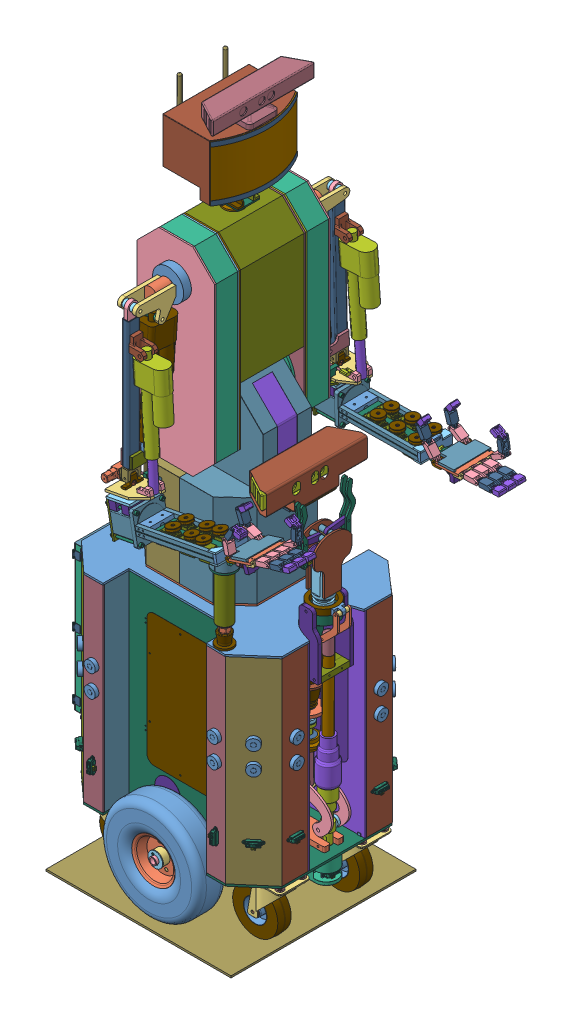
SolidWorks assembly sorbot, configuration По умолчанию. Lengths in mm. (continued)
Components (placement in the parent): (continued)
- pillar.10mm-9: pillar.10mm [Default] at (211.9932 95.4897 -58.2424) x (-0.73854 -0.67421 0) z (-0.67421 0.73854 0) size (7 10 7)
- pillar.10mm-10: pillar.10mm [Default] at (212.0094 150.4897 -58.2424) x (-0.73854 -0.67421 0) z (-0.67421 0.73854 0) size (7 10 7)
- platform.motor.drivers-1: platform.motor.drivers [Default] at (80.8907 152.4914 -189.9653) x (0 0 1) z (-1 0 0) size (159.34 76.47 117)
  - dirvers.motor.assembly-1: dirvers.motor.assembly [Default] at (49.223 64.9012 121.2019) size (145 32 117)
  - pillar.10mm-1: pillar.10mm [Default] at (-13.277 69.9012 103.7019) size (7 10 7)
  - vnh2sp30-1: vnh2sp30 [Default] at (2.7293 79.9012 115.4439) size (38 1.5 30)
  - pillar.10mm-2: pillar.10mm [Default] at (18.6548 69.9012 103.7019) size (7 10 7)
  - pillar.10mm-3: pillar.10mm [Default] at (18.6548 69.9012 127.4284) size (7 10 7)
  - pillar.10mm-4: pillar.10mm [Default] at (27.723 69.9012 103.7019) size (7 10 7)
  - vnh2sp30-2: vnh2sp30 [Default] at (43.7293 79.9012 115.4439) size (38 1.5 30)
  - pillar.10mm-5: pillar.10mm [Default] at (59.6548 69.9012 103.7019) size (7 10 7)
  - pillar.10mm-6: pillar.10mm [Default] at (59.6548 69.9012 127.4284) size (7 10 7)
  - pillar.10mm-7: pillar.10mm [Default] at (70.723 69.9012 103.7019) size (7 10 7)
  - vnh2sp30-3: vnh2sp30 [Default] at (86.7293 79.9012 115.4439) size (38 1.5 30)
  - pillar.10mm-8: pillar.10mm [Default] at (102.6548 69.9012 103.7019) size (7 10 7)
  - pillar.10mm-9: pillar.10mm [Default] at (102.6548 69.9012 127.4284) size (7 10 7)
  - fan1.fixture-1: fan1.fixture [Default] at (106.723 64.9012 93.8312) size (16.5 71.5 44)
  - PC Fan-1: PC Fan [Default] at (71.3146 136.8013 172.3383) x (0 -1 0) z (0 0 1) size (47.91 13.68 47.91)
    - Fan - housing-1: Fan - housing [Default] at (23.3881 57.9083 -56.6715) x (0 -1 0) z (-1 0 0) size (13.68 37 37)
    - Fan - propeller-1: Fan - propeller [Default] at (23.3881 58.6083 -56.6715) x (-0.764125 0 -0.645068) z (0 1 0) size (34 34 7.89)
  - radiator1-1: radiator1 [Default] at (2.2293 83.4012 115.4439) x (0 0 1) z (-1 0 0) size (47 23 17)
  - radiator2-1: radiator2 [Default] at (43.7293 83.4012 115.4439) x (0 0 1) z (-1 0 0) size (60 39 27)
  - radiator2-2: radiator2 [Default] at (86.7293 83.4012 115.4439) x (0 0 1) z (-1 0 0) size (60 39 27)
  - screw.m4x35-1: screw.m4x35 [Default] at (4.1241 64.9012 94.8432) size (10.8 29 10.8)
  - screw.m4x35-2: screw.m4x35 [Default] at (4.1241 64.9012 136.0446) size (10.8 29 10.8)
  - screw.m4x35-3: screw.m4x35 [Default] at (45.6241 64.9012 88.5829) size (10.8 29 10.8)
  - screw.m4x35-4: screw.m4x35 [Default] at (45.6241 64.9012 142.3048) size (10.8 29 10.8)
  - screw.m4x35-5: screw.m4x35 [Default] at (88.6241 64.9012 88.5829) size (10.8 29 10.8)
  - screw.m4x35-6: screw.m4x35 [Default] at (88.6241 64.9012 142.3048) size (10.8 29 10.8)
- computer.box.screw.fixture-5: computer.box.screw.fixture [Default] at (-89.5362 420.1505 8.4522) x (0 1 0) z (-1 0 0) size (25 10 10)
- computer.box.screw.fixture-6: computer.box.screw.fixture [Default] at (-89.5362 260.1505 8.4522) x (0 -1 0) z (1 0 0) size (25 10 10)
- computer.box.screw.fixture-7: computer.box.screw.fixture [Default] at (75.4638 420.1505 8.4522) x (0 -1 0) z (1 0 0) size (25 10 10)
- computer.box.screw.fixture-8: computer.box.screw.fixture [Default] at (75.4638 260.1505 8.4522) x (0 -1 0) z (1 0 0) size (25 10 10)
- computer.box.screw.fixture-9: computer.box.screw.fixture [Default] at (-7.0362 175.1505 8.4522) x (1 0 0) z (0 1 0) size (25 10 10)
- computer.box.screw.fixture-10: computer.box.screw.fixture [Default] at (-7.0362 505.1505 8.4522) x (1 0 0) z (0 1 0) size (25 10 10)
- computer.box.screw.fixture-11: computer.box.screw.fixture [Default] at (-6.9656 175.1505 -282.1821) x (1 0 0) z (0 -1 0) size (25 10 10)
- computer.box.screw.fixture-12: computer.box.screw.fixture [Default] at (75.5344 420.1505 -282.1821) x (0 1 0) z (1 0 0) size (25 10 10)
- computer.box.screw.fixture-13: computer.box.screw.fixture [Default] at (-6.9656 505.1505 -282.1821) x (1 0 0) z (0 -1 0) size (25 10 10)
- computer.box.screw.fixture-14: computer.box.screw.fixture [Default] at (75.5344 260.1505 -282.1821) x (0 1 0) z (1 0 0) size (25 10 10)
- computer.box.screw.fixture-15: computer.box.screw.fixture [Default] at (-89.4656 260.1505 -282.1821) x (0 1 0) z (1 0 0) size (25 10 10)
- computer.box.screw.fixture-16: computer.box.screw.fixture [Default] at (-89.4656 420.1505 -282.1821) x (0 1 0) z (1 0 0) size (25 10 10)
- plates.fixture-1: plates.fixture [Default] at (-94.2054 480.3702 -281.1821) x (0 0 1) z (-1 0 0) size (18.98 21 15)
- plates.fixture-2: plates.fixture [Default] at (-94.2054 228.5986 -281.1821) x (0 0 1) z (-1 0 0) size (18.98 21 15)
- left.plate-1: left.plate [Default] at (-11.6361 340.1505 -239.559) x (1 0 0) z (0 1 0) size (150 2 294)
- plates.fixture-3: plates.fixture [Default] at (-66.9634 476.3702 -242.559) x (0 0 -1) z (-1 0 0) size (18.98 21 15)
- plates.fixture-4: plates.fixture [Default] at (-66.9634 224.5986 -242.559) x (0 0 -1) z (-1 0 0) size (18.98 21 15)
- plate.console-1: plate.console [Default] at (-43.3033 477.3702 -231.7221) x (-0.961017 0 -0.276489) z (0.276489 0 -0.961017) size (44.8 2 28.3)
- plate.console-2: plate.console [Default] at (-43.3033 225.5986 -231.7221) x (-0.961017 0 -0.276489) z (0.276489 0 -0.961017) size (44.8 2 28.3)
- right.plate-1: right.plate [Default] at (-9.2671 340.1505 -29.4493) x (1 0 0) z (0 -1 0) size (150 2 294)
- plates.fixture-5: plates.fixture [Default] at (-109.2054 480.3702 7.4522) x (0 0 -1) z (1 0 0) size (18.98 21 15)
- plates.fixture-6: plates.fixture [Default] at (-109.2054 228.5986 7.4522) x (0 0 -1) z (1 0 0) size (18.98 21 15)
- plate.console-3: plate.console [Default] at (-37.759 479.3702 -31.8467) x (-0.993461 0 0.11417) z (0.11417 0 0.993461) size (44.8 2 28.3)
- plate.console-4: plate.console [Default] at (-37.759 227.5986 -31.8467) x (-0.993461 0 0.11417) z (0.11417 0 0.993461) size (44.8 2 28.3)
- plates.fixture-7: plates.fixture [Default] at (-79.5944 476.3702 -26.4493) x (0 0 1) z (1 0 0) size (18.98 21 15)
- plates.fixture-8: plates.fixture [Default] at (-79.5944 224.5986 -26.4493) x (0 0 1) z (1 0 0) size (18.98 21 15)
- us_sesnor_board-5: us_sesnor_board [Default] at (156.7984 270.4368 -340.1821) x (0 -1 0) z (-1 0 0) size (57 1.5 32)
- us_sesnor_board-6: us_sesnor_board [Default] at (208.5725 230.4368 -317.4683) x (0 1 0) z (0.759435 0 0.650583) size (57 1.5 32)
- us_sesnor_board-7: us_sesnor_board [Default] at (251.2324 210.4368 -249.3603) x (0 1 0) z (0.00186 0 0.999998) size (57 1.5 32)
- us_sesnor_board-8: us_sesnor_board [Default] at (251.1742 210.4368 -22.2417) x (0 1 0) z (0 0 1) size (57 1.5 32)
- us_sesnor_board-9: us_sesnor_board [Default] at (206.521 230.4368 45.4742) x (0 1 0) z (-0.759435 0 0.650583) size (57 1.5 32)
- us_sesnor_board-10: us_sesnor_board [Default] at (159.7428 270.4368 66.4522) x (0 -1 0) z (1 0 0) size (57 1.5 32)
- pillar.10mm-11: pillar.10mm [Default] at (143.5283 296.7164 -350.1821) x (0 -1 0) z (-1 0 0) size (7 10 7)
- pillar.10mm-12: pillar.10mm [Default] at (169.3356 244.6047 -350.1821) x (0 -1 0) z (-1 0 0) size (7 10 7)
- pillar.10mm-13: pillar.10mm [Default] at (225.1561 204.1572 -316.4293) x (0 1 0) z (0.759435 0 0.650583) size (7 10 7)
- pillar.10mm-14: pillar.10mm [Default] at (205.5571 256.2689 -333.2192) x (0 1 0) z (0.759435 0 0.650583) size (7 10 7)
- pillar.10mm-15: pillar.10mm [Default] at (261.2571 184.1572 -236.1088) x (0 1 0) z (0.00186 0 0.999998) size (7 10 7)
- pillar.10mm-16: pillar.10mm [Default] at (261.2091 236.2689 -261.9161) x (0 1 0) z (0.00186 0 0.999998) size (7 10 7)
- pillar.10mm-17: pillar.10mm [Default] at (261.1742 236.2689 -34.779) x (0 1 0) z (0 0 1) size (7 10 7)
- pillar.10mm-18: pillar.10mm [Default] at (261.1742 184.1572 -8.9716) x (0 1 0) z (0 0 1) size (7 10 7)
- pillar.10mm-19: pillar.10mm [Default] at (202.949 204.1572 61.7019) x (0 1 0) z (-0.759435 0 0.650583) size (7 10 7)
- pillar.10mm-20: pillar.10mm [Default] at (222.548 256.2689 44.9121) x (0 1 0) z (-0.759435 0 0.650583) size (7 10 7)
- pillar.10mm-21: pillar.10mm [Default] at (173.0129 296.7164 76.4522) x (0 -1 0) z (1 0 0) size (7 10 7)
- pillar.10mm-22: pillar.10mm [Default] at (147.2055 244.6047 76.4522) x (0 -1 0) z (1 0 0) size (7 10 7)
- acdc.220V.filter-1: acdc.220V.filter [Default] at (235.8821 406.6863 -46.2424) x (0 1 0) z (1 0 0) size (297.85 43 50)
- pillar.10mm-23: pillar.10mm [Default] at (235.8821 551.7681 -46.2424) x (0 -1 0) z (1 0 0) size (7 10 7)
- pillar.10mm-24: pillar.10mm [Default] at (235.8821 261.6046 -46.2424) x (-0.028691 -0.999588 0) z (0.999588 -0.028691 0) size (7 10 7)
- acdc.12v.power.supply-1: acdc.12v.power.supply [Default] at (169.7521 152.7755 -317.8791) x (0 1 0) z (0 0 -1) size (125 30 50)
- AC-DC-12-fixture-1: AC-DC-12-fixture [Default] at (138.7521 154.3322 -328.3791) x (0 0 1) z (0 1 0) size (24.5 56.75 30.18)
- AC-DC-12-fixture-2: AC-DC-12-fixture [Default] at (138.7521 154.3322 -307.3791) x (0 0 -1) z (0 -1 0) size (24.5 56.75 30.18)
- encoder-2-1: encoder-2 [Default] at (-6.6918 11.9368 -256.3681) x (1 0 0) z (0 -1 0) size (68 0.5 68)
- encoder-2-2: encoder-2 [Default] at (-6.6918 11.9368 -16.3681) x (1 0 0) z (0 -1 0) size (68 0.5 68)
- spool.220v-1: spool.220v [Default] at (27.3222 599.5624 89.7858) x (0 0 -1) z (0 -1 0) size (136.63 47 130)
  - spool.ac220v.base-1: spool.ac220v.base [Default] at (13.3335 111.5787 102.4119) size (136.63 5 130)
  - spool.220vac.spool.base.p1-1: spool.220vac.spool.base.p1 [Default] at (88.3335 116.5787 167.4119) size (121 5 121)
  - spool.disk.p1-1: spool.disk.p1 [Default] at (88.3335 121.5787 167.4119) size (121 1.5 121)
  - spool.disk2.pillar-1: spool.disk2.pillar [Default] at (141.3335 123.0787 167.4119) size (9 27 9)
  - spool.disk2.pillar-2: spool.disk2.pillar [Default] at (88.3335 123.0787 220.4119) size (9 27 9)
  - spool.disk2.pillar-3: spool.disk2.pillar [Default] at (35.3335 123.0787 167.4119) size (9 27 9)
  - spool.disk2.pillar-4: spool.disk2.pillar [Default] at (88.3335 123.0787 114.4119) size (9 27 9)
  - spool.disk.p2-1: spool.disk.p2 [Default] at (88.3335 150.0787 167.4119) size (121 1.5 121)
  - screw.m4x40-1: screw.m4x40 [Default] at (88.3335 118.5787 220.4119) x (-0.837169 0 -0.546944) z (-0.546944 0 0.837169) size (10 42 10)
  - screw.m4x40-2: screw.m4x40 [Default] at (141.3335 118.5787 167.4119) x (-0.837169 0 -0.546944) z (-0.546944 0 0.837169) size (10 42 10)
  - screw.m4x40-3: screw.m4x40 [Default] at (88.3335 118.5787 114.4119) x (-0.837169 0 -0.546944) z (-0.546944 0 0.837169) size (10 42 10)
  - screw.m4x40-4: screw.m4x40 [Default] at (35.3335 118.5787 167.4119) x (-0.837169 0 -0.546944) z (-0.546944 0 0.837169) size (10 42 10)
  - m4.nut-1: m4.nut [По умолчанию] at (141.3335 151.5787 167.4119) size (6.86 5 7.92)
  - m4.nut-2: m4.nut [По умолчанию] at (35.3335 151.5787 167.4119) size (6.86 5 7.92)
  - m4.nut-3: m4.nut [По умолчанию] at (88.3335 151.5787 114.4119) size (6.86 5 7.92)
  - m4.nut-4: m4.nut [По умолчанию] at (88.3335 151.5787 220.4119) size (6.86 5 7.92)
- wall2.cap-1: wall2.cap [Default] at (136.6115 375.4739 -212.2424) x (1 0 0) z (0 -1 0) size (170 0.5 350)
- wall2.cap-2: wall2.cap [Default] at (136.1134 375.6582 -62.2424) x (1 0 0) z (0 1 0) size (170 0.5 350)
- spool.220v.inlet-1: spool.220v.inlet [Default] at (160.9714 590.1505 61.3093) size (44 32.78 44)
- charger.module-1: charger.module [Default] at (132.5657 748.9564 17.9664) x (0.996526 0 -0.083283) z (0.083283 0 0.996526) size (60 284.68 60)
  - charger.module.base.p2-1: charger.module.base.p2 [Default] at (24.6973 28.3142 45.5581) size (59 10 59)
  - charger.module.case.p1-1: charger.module.case.p1 [Default] at (24.6973 38.3142 45.5581) size (59 22.9 59)
  - charger.module.camera-1: charger.module.camera [Default] at (24.6973 39.9144 45.5581) x (0.99995 0 0.009956) z (-0.009956 0 0.99995) size (34.64 19.2 34.64)
  - charger.module.motor.fixture-1: charger.module.motor.fixture [Default] at (24.6973 61.2142 45.5581) size (59 0.5 59)
  - charger.module.case.p2-1: charger.module.case.p2 [Default] at (24.6973 61.7142 45.5581) size (59 15 59)
  - charger.module.plug.p1-1: charger.module.plug.p1 [Default] at (24.6973 50.9902 45.5581) x (0.996646 0 0.081829) z (-0.081829 0 0.996646) size (32 40 32)
  - charger.module.motor-1: charger.module.motor [Default] at (46.1037 37.2096 54.3775) x (0.391862 0 -0.920024) z (0.920024 0 0.391862) size (12 35.5 10)
  - charger.module.gear.p1-1: charger.module.gear.p1 [Default] at (24.6973 67.2142 45.5581) x (0.999921 0 0.012536) z (-0.012536 0 0.999921) size (36.8 4.5 36.8)
  - charger.module.gear.p2-1: charger.module.gear.p2 [Default] at (46.1037 67.7096 54.3775) x (1 0 -0.000212) z (0.000212 0 1) size (11 8 11)
  - charger.module.insulation.p1-1: charger.module.insulation.p1 [Default] at (24.6973 63.7142 45.5581) x (0.996646 0 0.081829) z (-0.081829 0 0.996646) size (30 4 30)
  - charger.module.contact-1: charger.module.contact [Default] at (24.6973 58.7142 45.5581) size (30 5 30)
  - charger.module.insulation.p2-1: charger.module.insulation.p2 [Default] at (24.6973 56.7142 45.5581) x (0.996646 0 0.081829) z (-0.081829 0 0.996646) size (30 2 30)
  - charger.module.contact-2: charger.module.contact [Default] at (24.6973 51.7142 45.5581) size (30 5 30)
  - charger.module.insulation.p3-1: charger.module.insulation.p3 [Default] at (24.6973 49.2142 45.5581) size (30 2.5 30)
  - charger.module.cover-1: charger.module.cover [Default] at (24.6973 28.7142 45.5581) size (60 48 60)
  - charger.module.aluminum.base-1: charger.module.aluminum.base [Default] at (24.6973 23.3142 45.5581) size (59 32 59)
  - charger.module.handle-1: charger.module.handle [Default] at (24.6973 -104.6858 45.5581) size (40 128 40)
  - charger.module.cap-1: charger.module.cap [Default] at (24.6973 -107.1858 45.5581) size (38 14.5 38)
  - charger.module.cable.inlet.nut-1: charger.module.cable.inlet.nut [Default] at (24.6973 -104.6858 45.5581) x (0.829784 0 0.558085) z (-0.558085 0 0.829784) size (23.82 5 22.58)
  - charger.module.cable.inlet.nut.external-1: charger.module.cable.inlet.nut.external [Default] at (24.6973 -107.1858 45.5581) x (-0.837169 0 -0.546944) z (-0.546944 0 0.837169) size (25.34 15 22.82)
  - charger.module.cable.inlet.tail-1: charger.module.cable.inlet.tail [Default] at (24.6973 -114.1858 45.5581) x (-0.837169 0 -0.546944) z (-0.546944 0 0.837169) size (25.34 60 22.82)
- scanning.distance.meter.platform.bottom-1: scanning.distance.meter.platform.bottom [Default] at (253.6127 48.5992 -170.4978) x (-1 0 0) z (0 0 1) size (55.5 60.35 60)
  - servo.sm-s3317s-1: servo.sm-s3317s [Default] at (17.6103 2.1624 33.6342) size (42 32.4 16.3)
  - Sharp IR GP2D120-1: Sharp IR GP2D120 [Predeterminado] at (-1.2396 42.2544 36.8712) x (0 0 1) z (-1 0 0) size (44.5 19 13.9)
    - Sharp IR Body-1: Sharp IR Body [Predeterminado] at (-3.237 2.158 -6.95) size (44.5 13 13.9)
    - Sharp IR JST-1: Sharp IR JST [Predeterminado] at (-3.237 2.158 -3.95) size (28 18 7)
  - servo-sms3317s-lever-1: servo-sms3317s-lever [Default] at (9.4603 35.7624 33.6342) x (0 0 -1) z (-1 0 0) size (37.37 4.4 7)
  - scanning.distance.meter.sensor.fixture-1: scanning.distance.meter.sensor.fixture [Default] at (5.7103 36.1624 10.6342) size (7.5 15 46)
  - scanning.distance.meter.case-1: scanning.distance.meter.case [Default] at (11.0014 62.5124 33.6342) size (55.5 60.35 60)
- kinect-1: kinect [По умолчанию] at (202.8758 910.3423 -136.6669) x (0 0 1) z (-1 0 0) size (276 72 65)
- body.cover.glass-1: body.cover.glass [Default] at (129.0303 942.6564 -137.0438) x (0 0 1) z (-1 0 0) size (79.82 175.77 79.37)
- frontal.kinect.plate-1: frontal.kinect.plate [Default] at (172.5303 854.8423 -136.6669) x (0 0 -1) z (1 0 0) size (120 2 80)
- frontal.kinect.plate.fixture-1: frontal.kinect.plate.fixture [Default] at (134.0303 854.8423 -96.6669) x (0 1 0) z (1 0 0) size (40 20 66.5)
- frontal.kinect.plate.fixture-2: frontal.kinect.plate.fixture [Default] at (134.0303 854.8423 -196.6669) x (0 1 0) z (1 0 0) size (40 20 66.5)
- frontal.kinect.cover-1: frontal.kinect.cover [Default] at (172.5303 857.3423 -136.6669) x (0 0 -1) z (1 0 0) size (272 81 81)
- body.cover.back-1: body.cover.back [По умолчанию] at (-55.0648 1082.7934 -136.9735) x (0 0 1) z (-1 0 0) size (278.72 470.5 152.62)
- back.camera.housing-1: back.camera.housing [Default] at (-158.0178 1016.2961 -137.3735) x (0 0 1) z (-0.707107 -0.707107 0) size (92.1 36.15 55.95)
Mates (geometry in assembly coordinates):
- Концентричный1: concentric anti-aligned: cylinder of wheel-2/wheel.metal.internal-1 through (-6.6918 11.9368 -351.3681) axis (0 0 1) radius 10; cylinder of wheel-1/wheel.metal.internal-1 through (-6.6918 11.9368 79.1319) axis (0 0 -1) radius 10
- Концентричный2: concentric anti-aligned: cylinder of wheel-1/wheel.metal.internal-1 through (-6.6918 11.9368 79.1319) axis (0 0 -1) radius 10; cylinder of wheel.axis-1 through (-6.6918 11.9368 -361.8681) axis (0 0 1) radius 10
- Концентричный3: concentric anti-aligned: cylinder of wheel.axis-1 through (-6.6918 11.9368 -361.8681) axis (0 0 1) radius 10; cylinder of wheel.washer-1 through (-6.6918 11.9368 81.1319) axis (0 0 -1) radius 10
- Совпадение3: coincident anti-aligned: plane of wheel-1/wheel.metal.internal-1 through (-6.6918 11.9368 79.1319) normal (0 0 1); plane of wheel.washer-1 through (-6.6918 11.9368 79.1319) normal (0 0 -1)
- Концентричный4: concentric anti-aligned: cylinder of wheel.axis-1 through (-6.6918 11.9368 -361.8681) axis (0 0 1) radius 10; cylinder of wheel.washer-2 through (-6.6918 11.9368 -351.3681) axis (0 0 -1) radius 10
- Совпадение4: coincident anti-aligned: plane of wheel.washer-2 through (-6.6918 11.9368 -351.3681) normal (0 0 1); plane of wheel-2/wheel.metal.internal-1 through (-6.6918 11.9368 -351.3681) normal (0 0 -1)
- Параллельность1: parallel aligned: line of wheel.axis-1 through (0.9691 -6.5378 -355.8681) axis (-0.383049 0.923728 0); circle of wheel.axis.splint-2
- Концентричный5: concentric aligned: cylinder of wheel-2/wheel.metal.internal-1 through (-6.6918 11.9368 -291.3681) axis (0 0 -1) radius 19; cylinder of wheel.disk-1 through (-6.6918 11.9368 -311.3681) axis (0 0 -1) radius 18.9
- Совпадение7: coincident anti-aligned: plane of wheel-2/wheel.metal.internal-1 through (-25.4032 15.2361 -326.3681) normal (0 0 1); plane of wheel.disk-1 through (-6.6918 11.9368 -326.3681) normal (0 0 -1)
- Концентричный6: concentric anti-aligned: cylinder of wheel.axis-1 through (-6.6918 11.9368 -361.8681) axis (0 0 1) radius 10; cylinder of wheel.bearing-1 through (-6.6918 11.9368 -256.3681) axis (0 0 -1) radius 10
- Концентричный8: concentric aligned: cylinder of wheel.axis-1 through (-6.6918 11.9368 -361.8681) axis (0 0 1) radius 10; cylinder of wheel.stop.bearing-2/wheel.stop.bearing.p1-2 through (-6.6918 11.9368 -246.3457) axis (0 0 1) radius 10
- Совпадение10: coincident anti-aligned: plane of wheel.disk-1 through (-6.6918 11.9368 -256.3681) normal (0 0 1); plane of wheel.stop.bearing-2/wheel.stop.bearing.p1-1 through (-6.6918 11.9368 -256.3681) normal (0 0 -1)
- Концентричный10: concentric anti-aligned: cylinder of gearmotor-1 through (53.2168 119.2767 -284.0001) axis (0 0 1) radius 7; cylinder of gearmotor.sprocket.wheel.disk-1 through (53.2168 119.2767 -217.7117) axis (0 0 -1) radius 7
- Концентричный13: concentric anti-aligned: cylinder of wheel.axis-1 through (-6.6918 11.9368 -361.8681) axis (0 0 1) radius 10; cylinder of sprocket-1 through (-6.6918 11.9368 -268.3681) axis (0 0 -1) radius 26
- Концентричный14: concentric anti-aligned: circle of gearmotor-1; circle of sproket.initial-1
- Совпадение16: coincident aligned: plane of sproket.initial-1 through (64.3825 152.5534 -268.5001) normal (0 0 1); circle of gearmotor.sprocket.wheel.disk-1
- Параллельность2: parallel anti-aligned: plane of sproket.initial-1 through (64.3825 152.5534 -271.5001) normal (0 0 -1); plane of sprocket-1 through (4.6992 45.137 -268.3681) normal (0 0 1)
- Совпадение57: coincident anti-aligned: plane of sprocket-1 through (4.6992 45.137 -271.3681) normal (0 0 -1); plane of wheel.disk-1 through (-6.6918 11.9368 -271.3681) normal (0 0 1)
- Совпадение61: coincident anti-aligned: plane of gearmotor-1 through (53.2168 119.2767 -254.0001) normal (0 0 -1); plane of gearmotor.sprocket.wheel.disk-1 through (53.2168 119.2767 -254.0001) normal (0 0 1)
- Параллельность3: parallel aligned: plane of sproket.initial-1 through (64.3825 152.5534 -268.5001) normal (0 0 1); plane of sprocket-1 through (4.6992 45.137 -268.3681) normal (0 0 1)
- Совпадение65: coincident anti-aligned: plane of bottom-2 through (-49.3372 46.4368 -286.1821) normal (0 -1 0); plane of wheel.axis.frame-3 through (15.3082 46.4368 -205.8457) normal (0 1 0)
- Концентричный59: concentric anti-aligned: cylinder of wheel.axis-1 through (-6.6918 11.9368 -361.8681) axis (0 0 1) radius 10; cylinder of wheel.axis.frame-3 through (-6.6918 11.9368 -211.3457) axis (0 0 -1) radius 10
- Совпадение66: coincident anti-aligned: plane of wheel.stop.bearing-2/wheel.stop.bearing.p1-2 through (-6.6918 11.9368 -242.3457) normal (0 0 1); plane of wheel.axis.frame-3 through (-6.6918 11.9368 -242.3457) normal (0 0 -1)
- Совпадение68: coincident anti-aligned: plane of wheel.disk-2 through (-6.6918 11.9368 54.1319) normal (0 0 1); plane of wheel-1/wheel.metal.internal-1 through (11.3638 17.8524 54.1319) normal (0 0 -1)
- Концентричный60: concentric aligned: cylinder of wheel-1/wheel.metal.internal-1 through (-6.6918 11.9368 19.1319) axis (0 0 1) radius 19; cylinder of wheel.disk-2 through (-6.6918 11.9368 39.1319) axis (0 0 1) radius 18.9
- Концентричный62: concentric anti-aligned: cylinder of wheel.axis-1 through (-6.6918 11.9368 -361.8681) axis (0 0 1) radius 10; cylinder of wheel.bearing-2 through (-6.6918 11.9368 -8.8681) axis (0 0 -1) radius 10
- Совпадение69: coincident anti-aligned: plane of wheel.disk-2 through (-6.6918 11.9368 -8.8681) normal (0 0 -1); plane of wheel.bearing-2 through (-6.6918 11.9368 -8.8681) normal (0 0 1)
- Концентричный63: concentric aligned: cylinder of wheel.axis-1 through (-6.6918 11.9368 -361.8681) axis (0 0 1) radius 10; cylinder of wheel.stop.bearing-3/wheel.stop.bearing.p1-2 through (-6.6918 11.9368 -19.8681) axis (0 0 1) radius 10
- Совпадение70: coincident anti-aligned: plane of wheel.bearing-2 through (-6.6918 11.9368 -15.8681) normal (0 0 -1); plane of wheel.stop.bearing-3/wheel.stop.bearing.p1-2 through (-6.6918 11.9368 -15.8681) normal (0 0 1)
- Совпадение72: coincident anti-aligned: plane of wheel.axis.frame-4 through (-28.6918 46.4368 -66.3906) normal (0 1 0); plane of bottom-2 through (-49.3372 46.4368 -286.1821) normal (0 -1 0)
- Совпадение73: coincident anti-aligned: plane of wheel.axis.frame-4 through (-6.6918 11.9368 -29.8906) normal (0 0 1); plane of wheel.stop.bearing-3/wheel.stop.bearing.p1-1 through (-6.6918 11.9368 -29.8906) normal (0 0 -1)
- Концентричный65: concentric aligned: cylinder of wheel.axis-1 through (-6.6918 11.9368 -361.8681) axis (0 0 1) radius 10; cylinder of wheel.axis.frame-4 through (-6.6918 11.9368 -60.8906) axis (0 0 1) radius 10
- Совпадение74: coincident anti-aligned: plane of wheel.disk-2 through (-6.6918 11.9368 -0.8681) normal (0 0 -1); plane of sprocket-2 through (4.3334 45.2603 -0.8681) normal (0 0 1)
- Концентричный66: concentric anti-aligned: cylinder of wheel.disk-2 through (-6.6918 11.9368 -15.8681) axis (0 0 1) radius 26.5; cylinder of sprocket-2 through (-6.6918 11.9368 -0.8681) axis (0 0 -1) radius 26
- Концентричный67: concentric anti-aligned: cylinder of gearmotor-2 through (-40.8776 119.0545 10.8308) axis (0 0 -1) radius 7; cylinder of gearmotor.sprocket.wheel.disk-2 through (-40.8776 119.0545 -55.4577) axis (0 0 1) radius 7
- Совпадение77: coincident anti-aligned: plane of gearmotor.sprocket.wheel.disk-2 through (-40.8776 119.0545 -19.1692) normal (0 0 -1); plane of gearmotor-2 through (-40.8776 119.0545 -19.1692) normal (0 0 1)
- Совпадение78: coincident anti-aligned: plane of gearmotor-2 through (-39.033 127.9382 4.8308) normal (0.999846 0.017524 0); plane of gearmotor.sprocket.wheel.disk-2 through (-39.033 127.9382 -55.4577) normal (-0.999846 -0.017524 0)
- Совпадение79: coincident anti-aligned: plane of sproket.initial-2 through (-52.3821 152.2156 -4.6692) normal (0 0 -1); plane of gearmotor.sprocket.wheel.disk-2 through (-40.8776 119.0545 -4.6692) normal (0 0 1)
- Концентричный68: concentric anti-aligned: circle of gearmotor.sprocket.wheel.disk-2; circle of sproket.initial-2
- Концентричный69: concentric aligned: cylinder of wheel.axis-1 through (-6.6918 11.9368 -361.8681) axis (0 0 1) radius 10; cylinder of wheel.disk-2 through (-6.6918 11.9368 39.1319) axis (0 0 1) radius 18.9
- Заблокировать1: lock: unknown of wheel.washer-1; unknown of wheel.disk-2
- Заблокировать3: lock: unknown of sproket.initial-1; unknown of gearmotor.sprocket.wheel.disk-1
- Заблокировать4: lock: unknown of gearmotor-2; unknown of gearmotor.sprocket.wheel.disk-2
- Совпадение81: coincident anti-aligned: plane of wheel.disk-1 through (-6.6918 11.9368 -263.3681) normal (0 0 1); plane of wheel.bearing-1 through (-6.6918 11.9368 -263.3681) normal (0 0 -1)
- Концентричный77: concentric anti-aligned: cylinder of gearmotor-2 through (-40.8776 119.0545 -257.1692) axis (0 0 1) radius 32.5; cylinder of gearmotor.fixture.p3-1 through (-40.8776 119.0545 -181.1702) axis (0 0 -1) radius 32.4
- Концентричный80: concentric anti-aligned: cylinder of gearmotor-1 through (53.2168 119.2767 -250.0001) axis (0 0 1) radius 20; cylinder of gearmotor.fixture.p2-3 through (53.2168 119.2767 -237.0001) axis (0 0 -1) radius 21.5
- Совпадение104: coincident anti-aligned: plane of gearmotor-1 through (53.2168 119.2767 -245.0001) normal (0 0 -1); plane of gearmotor.fixture.p2-3 through (10.2084 53.4933 -245.0001) normal (0 0 1)
- Параллельность25: parallel aligned: line of bottom-2 through (267.1742 51.9368 11.9714) axis (0 0 -1); line of wall1-1 through (26.1889 166.4368 -62.2424) axis (0 0 -1)
- Совпадение111: coincident aligned: line of wall1-1 through (21.1889 585.1505 -212.2424) axis (0 -1 0); line of wall2-2 through (21.1889 585.1505 -212.2424) axis (0 -1 0)
- Совпадение114: coincident anti-aligned: plane of wall2-2 through (21.1889 831.1682 -212.2424) normal (0 0 1); plane of wall3-1 through (107.1741 171.4368 -212.2424) normal (0 0 -1)
- Совпадение116: coincident aligned: line of wall2-2 through (107.1741 51.9368 -216.2424) axis (0 1 0); line of wall4-1 through (107.1741 51.4368 -216.2424) axis (0 1 0)
- Совпадение117: coincident anti-aligned: plane of wall2-2 through (107.1741 -108.1132 -212.2424) normal (-1 0 0); plane of wall4-1 through (107.1741 51.4368 -56.2424) normal (1 0 0)
- Совпадение120: coincident anti-aligned: plane of wall2-1 through (21.1889 831.1682 -58.2424) normal (0 0 1); plane of wall6-1 through (263.1742 655.3334 -58.2424) normal (0 0 -1)
- Совпадение121: coincident anti-aligned: plane of bottom-2 through (-49.3372 51.9368 -286.1821) normal (0 1 0); plane of wall6-1 through (263.1742 51.9368 -58.2424) normal (0 -1 0)
- Совпадение122: coincident aligned: line of bottom-2 through (267.1742 51.9368 11.9714) axis (0 0 -1); line of wall6-1 through (267.1742 51.9368 11.8264) axis (0 0 -1)
- Параллельность26: parallel aligned: line of bottom-2 through (184.9009 51.9368 82.4522) axis (0.759435 0 -0.650583); line of wall7-1 through (184.8921 51.9368 82.4377) axis (0.759435 0 -0.650583)
- Совпадение127: coincident anti-aligned: plane of bottom-2 through (-49.3372 51.9368 -286.1821) normal (0 1 0); plane of wall7-1 through (263.5537 51.9368 9.7838) normal (0 -1 0)
- Совпадение142: coincident anti-aligned: plane of bottom-2 through (-49.3372 51.9368 -286.1821) normal (0 1 0); plane of wall8-2 through (132.798 51.9368 -356.1821) normal (0 -1 0)
- Совпадение144: coincident anti-aligned: plane of bottom-2 through (-49.3372 51.9368 -286.1821) normal (0 1 0); plane of wall9-1 through (132.9009 51.9368 78.4522) normal (0 -1 0)
- Совпадение145: coincident aligned: line of bottom-2 through (132.9009 51.9368 12.4522) axis (0 0 1); line of wall9-1 through (132.9009 51.9368 8.55) axis (0 0 1)
- Совпадение146: coincident aligned: line of bottom-2 through (39.4201 51.9368 12.4522) axis (1 0 0); line of wall10-1 through (-146.6756 51.9368 12.4522) axis (1 0 0)
- Совпадение147: coincident anti-aligned: plane of wall9-1 through (132.9009 655.1671 8.55) normal (-1 0 0); plane of wall10-1 through (132.9009 864.7556 8.4522) normal (1 0 0)
- Совпадение149: coincident anti-aligned: plane of bottom-2 through (-49.3372 51.9368 -286.1821) normal (0 1 0); plane of wall9-2 through (-150.6756 51.9368 78.5322) normal (0 -1 0)
- Совпадение157: coincident anti-aligned: line of wall3-1 through (107.1741 166.4368 -62.2424) axis (0 0 -1); line of wall4-1 through (107.1741 166.4368 -216.2424) axis (0 0 1)
- Совпадение161: coincident anti-aligned: line of wall2-2 through (21.1889 166.4368 -212.2424) axis (1 0 0); line of wall3-1 through (107.1741 166.4368 -212.2424) axis (-1 0 0)
- Совпадение162: coincident anti-aligned: line of wall2-1 through (107.1741 166.4368 -62.2424) axis (-1 0 0); line of wall3-1 through (26.1889 166.4368 -62.2424) axis (1 0 0)
- Совпадение170: coincident anti-aligned: plane of bottom-2 through (-49.3372 51.9368 -286.1821) normal (0 1 0); plane of wall7-v1-1 through (-149.98 51.9368 -93.7194) normal (0 -1 0)
- Параллельность29: parallel anti-aligned: line of bottom-2 through (-275.9596 51.9368 11.9714) axis (0.73854 0 0.67421); line of wall7-v1-1 through (-199.0366 51.9368 82.0998) axis (-0.73854 0 -0.67421)
- Совпадение174: coincident anti-aligned: line of wall7-v1-1 through (-275.9003 51.9368 11.9312) axis (0 1 0); line of wall11-1 through (-275.9003 585.1505 11.9312) axis (0 -1 0)
- Совпадение182: coincident anti-aligned: plane of bottom-2 through (-49.3372 51.9368 -286.1821) normal (0 1 0); plane of wall9-3 through (-150.7539 51.9368 -286.2798) normal (0 -1 0)
- Совпадение184: coincident anti-aligned: plane of bottom-2 through (-49.3372 51.9368 -286.1821) normal (0 1 0); plane of wall10-v1-1 through (132.8227 51.9368 -286.1821) normal (0 -1 0)
- Совпадение188: coincident anti-aligned: plane of bottom-2 through (-49.3372 51.9368 -286.1821) normal (0 1 0); plane of wall9-4 through (132.8227 51.9368 -286.2798) normal (0 -1 0)
- Совпадение191: coincident anti-aligned: line of bottom-2 through (184.9009 51.9368 -356.1821) axis (-1 0 0); line of wall8-2 through (132.798 51.9368 -356.1821) axis (1 0 0)
- Совпадение201: coincident anti-aligned: plane of bottom-2 through (-49.3372 51.9368 -286.1821) normal (0 1 0); plane of wall7-3 through (183.3311 51.9368 -352.2595) normal (0 -1 0)
- Параллельность33: parallel aligned: line of bottom-2 through (267.1742 51.9368 -285.7013) axis (-0.759435 0 -0.650583); line of wall7-3 through (267.1973 51.9368 -285.6811) axis (-0.759435 0 -0.650583)
- Параллельность52: parallel anti-aligned: plane of gearmotor-3 through (-22.0648 623.1505 -128.1055) normal (-1 0 0); plane of turret-1/turret-p1-1 through (-22.0648 627.1934 -130.2473) normal (1 0 0)
- Концентричный93: concentric aligned: cylinder of gearmotor-3 through (-20.0648 629.1505 -136.9555) axis (0 -1 0) radius 7; cylinder of turret-1/turret-p1-1 through (-20.0648 627.1934 -136.9555) axis (0 -1 0) radius 7
- Концентричный110: concentric anti-aligned: cylinder of bolt1-2 through (172.9115 63.0264 3.3236) axis (0 -1 0) radius 5; cylinder of bolt1.nut-9 through (172.9115 51.9368 3.3236) axis (0 1 0) radius 5
- Концентричный111: concentric anti-aligned: cylinder of turret-1/turret-p1-1 through (-20.0648 603.2934 -136.9555) axis (0 1 0) radius 74; cylinder of turret.table-1 through (-20.0648 612.7934 -136.9555) axis (0 -1 0) radius 35
- Концентричный112: concentric aligned: cylinder of gearmotor-3 through (-20.0648 629.1505 -136.9555) axis (0 -1 0) radius 7; cylinder of turret.center-1 through (-20.0648 622.7934 -136.9555) axis (0 -1 0) radius 7
- Совпадение223: coincident anti-aligned: plane of turret-1/turret-p1-1 through (-20.0648 607.7934 -136.9555) normal (0 1 0); plane of turret.center-1 through (-20.0648 607.7934 -136.9555) normal (0 -1 0)
- Совпадение230: coincident anti-aligned: plane of gearmotor.fixture.p2-3 through (10.2084 53.4933 -245.0001) normal (0 1 0); plane of wheel.axis.frame.fixture.p2-3 through (-51.698 53.4933 -213.5833) normal (0 -1 0)
- Совпадение236: coincident anti-aligned: plane of bottom-2 through (-49.3372 51.9368 -286.1821) normal (0 1 0); plane of wall-fixture-3-2 through (213.2226 51.9368 -31.5478) normal (0 -1 0)
- Совпадение242: coincident anti-aligned: plane of gearmotor-2 through (-40.8776 119.0545 -28.1692) normal (0 0 1); plane of gearmotor.fixture.p2.1-1 through (2.1309 53.4368 -28.1692) normal (0 0 -1)
- Совпадение246: coincident anti-aligned: plane of bottom-2 through (-49.3372 51.9368 -286.1821) normal (0 1 0); plane of wheel.axis.frame.fixture.p2-1 through (43.2929 51.9368 -36.1421) normal (0 -1 0)
- Совпадение248: coincident anti-aligned: plane of wheel.axis.frame-4 through (15.3082 32.4368 -66.3906) normal (0 -1 0); plane of wheel.axis.frame.fixture.p1-1 through (42.6901 32.4368 -36.0198) normal (0 1 0)
- Концентричный116: concentric aligned: circle of wheel.axis.frame.fixture.p1-1; circle of wheel.axis.frame.fixture.p2-1
- Совпадение252: coincident anti-aligned: plane of wall7-v1-1 through (-271.8817 585.1505 10.1837) normal (0 1 0); plane of cap-1 through (216.6678 585.1505 -83.5666) normal (0 -1 0)
- Совпадение253: coincident anti-aligned: plane of cap-1 through (216.6678 590.1505 -83.5666) normal (0 1 0); plane of turret-1/turret-p4-1 through (-19.4709 590.1505 -137.0226) normal (0 -1 0)
- Совпадение254: coincident anti-aligned: plane of turret-1/turret-p1-1 through (-20.0648 607.7934 -136.9555) normal (0 1 0); plane of turret.table-1 through (-20.0648 607.7934 -360.2969) normal (0 -1 0)
- Заблокировать30: lock: unknown of ?; unknown of bolt1-15
- Заблокировать31: lock: unknown of ?; unknown of bolt1-15
- Заблокировать32: lock: unknown of bolt1-15; unknown of bolt1.nut-6
- Заблокировать33: lock: unknown of ?; unknown of bolt1-16
- Заблокировать34: lock: unknown of ?; unknown of bolt1-16
- Заблокировать35: lock: unknown of bolt1-16; unknown of bolt1.nut-5
- Заблокировать36: lock: unknown of ?; unknown of bolt1-13
- Заблокировать37: lock: unknown of ?; unknown of bolt1-13
- Заблокировать38: lock: unknown of bolt1-13; unknown of bolt1.nut-7
- Заблокировать39: lock: unknown of ?; unknown of bolt1-14
- Заблокировать40: lock: unknown of ?; unknown of bolt1-14
- Заблокировать41: lock: unknown of bolt1-14; unknown of bolt1.nut-8
- Совпадение276: coincident anti-aligned: plane of bottom-2 through (-49.3372 51.9368 -286.1821) normal (0 1 0); plane of wall-fixture-3-3-1 through (-242.5877 51.9368 -17.2349) normal (0 -1 0)
- Совпадение277: coincident anti-aligned: plane of wall7-v1-1 through (-271.8817 -52.2153 10.1837) normal (0.67421 0 -0.73854); plane of wall-fixture-3-3-1 through (-269.5561 51.9368 12.3067) normal (-0.67421 0 0.73854)
- Заблокировать42: lock: unknown of ?; unknown of bolt1-11
- Заблокировать43: lock: unknown of ?; unknown of bolt1-10
- Заблокировать44: lock: unknown of ?; unknown of bolt1-9
- Заблокировать45: lock: unknown of ?; unknown of bolt1-12
- Заблокировать46: lock: unknown of ?; unknown of bolt1-11
- Заблокировать47: lock: unknown of ?; unknown of bolt1-10
- Заблокировать48: lock: unknown of ?; unknown of bolt1-9
- Заблокировать49: lock: unknown of ?; unknown of bolt1-12
- Заблокировать50: lock: unknown of bolt1-11; unknown of bolt1.nut-1
- Заблокировать51: lock: unknown of bolt1-10; unknown of bolt1.nut-4
- Заблокировать52: lock: unknown of bolt1-9; unknown of bolt1.nut-3
- Заблокировать53: lock: unknown of bolt1-12; unknown of bolt1.nut-2
- Совпадение282: coincident anti-aligned: plane of bottom-2 through (-49.3372 51.9368 -286.1821) normal (0 1 0); plane of bolt1.nut-1 through (-189.5596 51.9368 -278.9161) normal (0 -1 0)
- Заблокировать54: lock: unknown of ?; unknown of bolt1-1
- Заблокировать55: lock: unknown of ?; unknown of bolt1-3
- Заблокировать56: lock: unknown of ?; unknown of bolt1-2
- Заблокировать57: lock: unknown of ?; unknown of bolt1-4
- Заблокировать58: lock: unknown of ?; unknown of bolt1-1
- Заблокировать59: lock: unknown of ?; unknown of bolt1-3
- Заблокировать60: lock: unknown of ?; unknown of bolt1-2
- Заблокировать61: lock: unknown of ?; unknown of bolt1-4
- Заблокировать62: lock: unknown of bolt1-3; unknown of bolt1.nut-10
- Заблокировать63: lock: unknown of bolt1-1; unknown of bolt1.nut-11
- Заблокировать64: lock: unknown of bolt1-2; unknown of bolt1.nut-9
- Заблокировать65: lock: unknown of bolt1-4; unknown of bolt1.nut-12
- Совпадение287: coincident anti-aligned: plane of bottom-2 through (-49.3372 51.9368 -286.1821) normal (0 1 0); plane of bolt1.nut-9 through (180.9944 51.9368 3.3236) normal (0 -1 0)
- Заблокировать66: lock: unknown of ?; unknown of bolt1-7
- Заблокировать67: lock: unknown of ?; unknown of bolt1-7
- Заблокировать68: lock: unknown of ?; unknown of bolt1-6
- Заблокировать69: lock: unknown of ?; unknown of bolt1-8
- Заблокировать70: lock: unknown of ?; unknown of bolt1-6
- Заблокировать71: lock: unknown of ?; unknown of bolt1-8
- Заблокировать72: lock: unknown of bolt1-7; unknown of bolt1.nut-13
- Заблокировать73: lock: unknown of bolt1-6; unknown of bolt1.nut-15
- Заблокировать75: lock: unknown of bolt1-5; unknown of bolt1.nut-14
- Заблокировать76: lock: unknown of bolt1-8; unknown of bolt1.nut-16
- Заблокировать77: lock: unknown of ?; unknown of bolt1-5
- Совпадение290: coincident anti-aligned: plane of bottom-2 through (-49.3372 51.9368 -286.1821) normal (0 1 0); plane of bolt1.nut-13 through (164.6729 51.9368 -277.7529) normal (0 -1 0)
- Касательный1: tangent anti-aligned: cylinder of wheel-1/wheel.chamber-1 through (-6.6918 11.9368 97.7637) axis (0 0 -1) radius 135; plane of ground-1 through (232.7402 -123.0632 115.6816) normal (0 1 0)
- Концентричный125: concentric aligned: cylinder of body.center-1 through (-20.0648 982.0246 -136.9555) axis (0 -1 0) radius 11; cylinder of body_pivot_fixture-1 through (-20.0648 962.0246 -136.9555) axis (0 -1 0) radius 11
- Концентричный163: concentric aligned: cylinder of body_axis-1 through (-20.0648 1016.5246 -50.7475) axis (0 0 -1) radius 10.9; cylinder of body.frame.p1.fixture-2 through (-20.0648 1016.5246 -209.3595) axis (0 0 -1) radius 10.9
- Заблокировать91: lock: unknown of body_axis-1; unknown of body.frame.p1.fixture-2
- Параллельность60: parallel aligned: cylinder of arm.actuator-1/arm.actuator.p1-1 through (-88.8064 993.1542 1.2558) axis (0 0 -1) radius 4.1; cylinder of arm.actuator.p2-1 through (-61.0144 1401.6056 11.2558) axis (0 0 -1) radius 4
- Концентричный165: concentric anti-aligned: cylinder of arm.actuator-1/arm.actuator.p1-1 through (-79.7097 1126.8451 -13.7442) axis (0.067885 0.997693 0) radius 10; cylinder of arm.actuator.p2-1 through (-60.4374 1410.086 -13.7442) axis (-0.067885 -0.997693 0) radius 10
- Концентричный454: concentric: cylinder of ? through (-88.5767 993.1387 1.2558) axis (0 0 -1) radius 4.1; cylinder of arm.lift.actuator.fixture.p2-1 through (-88.5767 993.1387 15.1693) axis (0 0 -1) radius 4
- Касательный32: tangent anti-aligned: cylinder of arm.actuator-1/arm.actuator.p1-1 through (-89.3495 985.1727 -13.7442) axis (0.067885 0.997693 0) radius 10; plane of arm.lift.actuator.fixture.p3-1 through (-88.5767 993.1387 -3.7442) normal (0 0 -1)
- Концентричный176: concentric aligned: cylinder of arm.actuator.p2-1 through (-61.0144 1401.6056 11.2558) axis (0 0 -1) radius 4; cylinder of shoulder.p4-1 through (-61.0144 1401.6056 -23.7442) axis (0 0 -1) radius 4
- Концентричный179: concentric aligned: cylinder of arm.actuator.p2-1 through (-61.0144 1401.6056 11.2558) axis (0 0 -1) radius 4; cylinder of shoulder.p4-2 through (-61.0144 1401.6056 0.2558) axis (0 0 -1) radius 4
- Концентричный183: concentric aligned: cylinder of arm.lift.actuator.fixture.p2-1 through (-88.5767 993.1387 15.1693) axis (0 0 -1) radius 4; cylinder of arm.lift.actuator.fixture.p3-1 through (-88.5767 993.1387 15.2558) axis (0 0 -1) radius 4
- Касательный11: tangent anti-aligned: cylinder of arm.actuator.p2-1 through (-60.4422 1410.0864 -13.7442) axis (-0.067324 -0.997731 0) radius 10; plane of shoulder.p4-2 through (-59.9468 1400.1462 -3.7442) normal (0 0 -1)
- Касательный12: tangent anti-aligned: cylinder of arm.actuator.p2-1 through (-60.4374 1410.086 -13.7442) axis (-0.067885 -0.997693 0) radius 10; plane of shoulder.p4-1 through (-59.9469 1400.1462 -23.7442) normal (0 0 1)
- Заблокировать105: lock: unknown of shoulder.p4-1; unknown of shoulder.p6-1
- Заблокировать106: lock: unknown of shoulder.p4-2; unknown of shoulder.p6-2
- Концентричный203: concentric anti-aligned: cylinder of arm.actuator-2/arm.actuator.p1-1 through (-12.7848 1153.0007 89.4303) axis (0 -0.997661 0.068351) radius 10; cylinder of arm.actuator.p2-2 through (-12.7848 967.3083 102.1523) axis (0 0.997661 -0.068351) radius 10
- Концентричный217: concentric anti-aligned: cylinder of arm.actuator100mm.p2-1 through (49.2564 930.6158 140.2746) axis (-0.061067 0.998134 0) radius 10; cylinder of arm.actuator100mm..p1-1 through (35.0693 1162.5008 140.2746) axis (0.061067 -0.998134 0) radius 10
- Параллельность77: parallel anti-aligned: cylinder of arm.actuator100mm..p1-1 through (29.8176 1248.3403 125.2746) axis (0 0 1) radius 4; cylinder of arm.actuator100mm.p2-1 through (48.7373 939.0999 165.2746) axis (0 0 -1) radius 4
- Заблокировать111: lock: unknown of ?; unknown of arm.actuator.p2-2
- Заблокировать161: lock: unknown of ?; unknown of arm.actuator.p2-1
- Концентричный281: concentric anti-aligned: cylinder of cap-hinge-1 through (95.4017 1325.4557 -46.5922) axis (0 -1 0) radius 2; cylinder of cap-hinge-p1-1 through (95.4017 1286.2182 -46.5922) axis (0 1 0) radius 2
- Совпадение460: coincident anti-aligned: plane of cap-hinge-1 through (75.4017 1315.4557 -52.4258) normal (0 -1 0); plane of cap-hinge-p1-1 through (75.4017 1315.4557 -51.5352) normal (0 1 0)
- Совпадение462: coincident anti-aligned: plane of arm.p1.m-1 through (-3.763 964.7884 152.9102) normal (1 0 0); plane of actuator.100.fixture-1 through (-3.763 1277.5198 127.4102) normal (-1 0 0)
- Совпадение463: coincident anti-aligned: line of arm.p1.m-1 through (-3.763 964.7884 127.4102) axis (0 1 0); line of actuator.100.fixture-1 through (-3.763 1277.5198 127.4102) axis (0 -1 0)
- Касательный17: tangent anti-aligned: cylinder of arm.actuator100mm..p1-1 through (29.329 1256.3254 140.2746) axis (0.061067 -0.998134 0) radius 10; plane of actuator.100.fixture-1 through (40.237 1209.783 150.2746) normal (0 0 -1)
- Концентричный291: concentric aligned: cylinder of arm.actuator100mm..p1-1 through (29.8176 1248.3403 125.2746) axis (0 0 1) radius 4; cylinder of actuator.100.fixture-1 through (29.8176 1248.3403 120.1602) axis (0 0 1) radius 4
- Заблокировать187: lock: unknown of arm.p1.m-1; unknown of actuator.100.fixture-1
- Заблокировать188: lock: unknown of arm.p1.m-1; unknown of forearm.rotate.p9-1
- Заблокировать122: lock: unknown of arm.actuator100mm..p1-1; unknown of arm.actuator100mm.p2-1
- Концентричный297: concentric aligned: cylinder of arm.actuator.p2-2 through (12.2152 975.7884 101.5713) axis (-1 0 0) radius 4; cylinder of forearm.rotate.p12-1 through (-21.7679 975.7884 101.5713) axis (-1 0 0) radius 4
- Совпадение470: coincident: unknown of arm.p1.m-1; unknown of forearm.rotate.p12-1
- Заблокировать196: lock: unknown of arm.p1.m-1; unknown of forearm.rotate.p12-1
- Заблокировать207: lock: unknown of lower.arm.p2-3; unknown of lower.arm.p3-1
- Заблокировать208: lock: unknown of lower.arm.p2-1; unknown of lower.arm.p3-1
- Заблокировать216: lock: unknown of lower.arm.p3-1; unknown of ?
- Заблокировать217: lock: unknown of lower.arm.p3-1; unknown of ?
- Заблокировать218: lock: unknown of lower.arm.p3-1; unknown of ?
- Заблокировать219: lock: unknown of lower.arm.p3-1; unknown of ?
- Заблокировать220: lock: unknown of lower.arm.p3-1; unknown of ?
- Заблокировать221: lock: unknown of lower.arm.p3-1; unknown of ?
- Концентричный317: concentric anti-aligned: cylinder of HS-311 Hitec Standard Servo and Horn-1/HS-311-p2-1 through (119.3969 887.1533 157.9974) axis (-0.185706 0.982605 0) radius 4.064; cylinder of lower.arm.p9-1 through (118.2362 893.2946 157.9974) axis (0.185706 -0.982605 0) radius 12
- Совпадение569: coincident anti-aligned: plane of HS-311 Hitec Standard Servo and Horn-1/HS-311-p2-1 through (120.3857 893.7008 149.5983) normal (-0.185706 0.982605 0); plane of lower.arm.p9-1 through (118.2362 893.2946 157.9974) normal (0.185706 -0.982605 0)
- Заблокировать244: lock: unknown of ?; unknown of lower.arm.p9-1
- Концентричный318: concentric aligned: cylinder of HS-311 Hitec Standard Servo and Horn-3/HS-311-p2-1 through (119.3969 887.1533 122.4974) axis (-0.185706 0.982605 0) radius 4.064; cylinder of lower.arm.p9-2 through (119.1648 888.3816 122.4974) axis (-0.185706 0.982605 0) radius 4
- Концентричный319: concentric aligned: cylinder of HS-311 Hitec Standard Servo and Horn-2/HS-311-p2-1 through (173.4402 897.3672 119.9974) axis (-0.185706 0.982605 0) radius 4.064; cylinder of lower.arm.p9-5 through (173.2081 898.5954 119.9974) axis (-0.185706 0.982605 0) radius 4
- Концентричный320: concentric aligned: cylinder of HS-311 Hitec Standard Servo and Horn-4/HS-311-p2-1 through (207.1632 903.7406 117.4346) axis (-0.185706 0.982605 0) radius 4.064; cylinder of lower.arm.p9-6 through (206.9311 904.9689 117.4346) axis (-0.185706 0.982605 0) radius 4
- Концентричный321: concentric aligned: cylinder of HS-311 Hitec Standard Servo and Horn-5/HS-311-p2-1 through (173.4402 897.3672 160.9974) axis (-0.185706 0.982605 0) radius 4.064; cylinder of lower.arm.p9-4 through (173.2081 898.5954 160.9974) axis (-0.185706 0.982605 0) radius 4
- Концентричный322: concentric aligned: cylinder of HS-311 Hitec Standard Servo and Horn-6/HS-311-p2-1 through (207.1632 903.7406 163.1146) axis (-0.185706 0.982605 0) radius 4.064; cylinder of lower.arm.p9-3 through (206.9311 904.9689 163.1146) axis (-0.185706 0.982605 0) radius 4
- Совпадение570: coincident anti-aligned: plane of HS-311 Hitec Standard Servo and Horn-5/HS-311-p2-1 through (174.429 903.9147 152.5983) normal (-0.185706 0.982605 0); plane of lower.arm.p9-4 through (172.2795 903.5084 160.9974) normal (0.185706 -0.982605 0)
- Совпадение571: coincident anti-aligned: plane of HS-311 Hitec Standard Servo and Horn-6/HS-311-p2-1 through (203.8531 909.4756 171.5136) normal (-0.185706 0.982605 0); plane of lower.arm.p9-3 through (206.0025 909.8819 163.1146) normal (0.185706 -0.982605 0)
